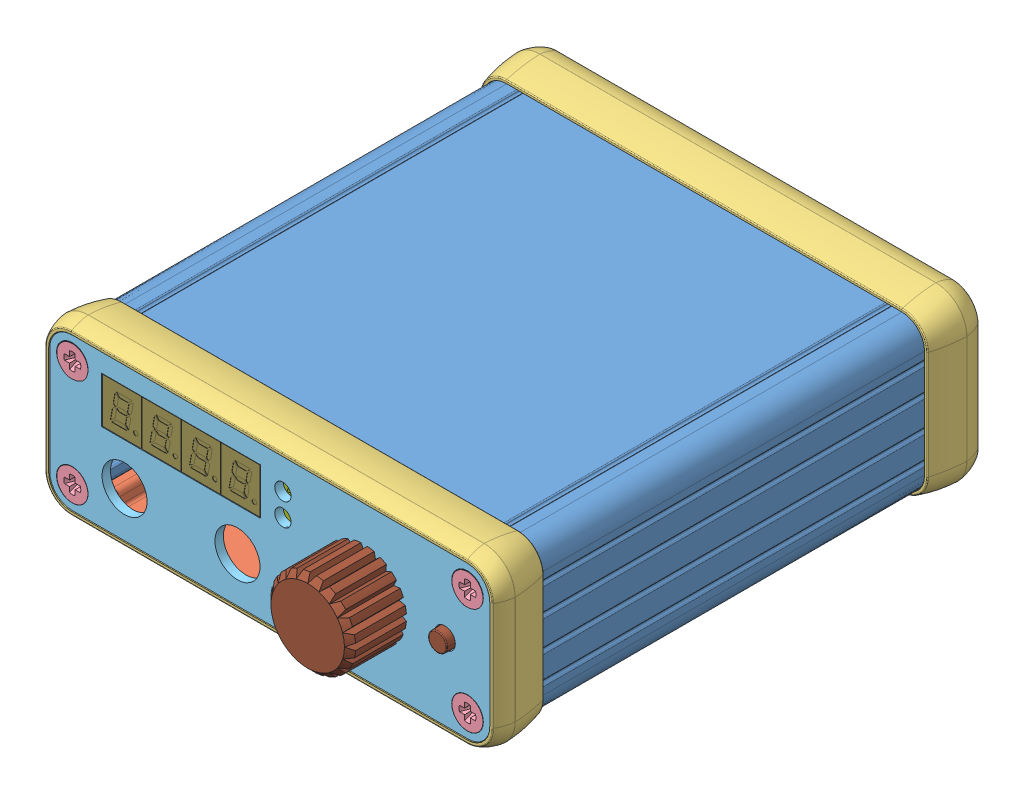
SolidWorks assembly Assembly_microbench_psu, configuration Standard. Lengths in mm. (continued)
Components (placement in the parent): (continued)
- main-board.step-1: main-board.step [Standard] at (-93.8915 -23.4474 -41.4) x (0 0 1) z (0 1 0) size (82.8 75 12.43) (continued)
  - C208.step-1: C208.step [Standard] at origin size (0.65 1.15 0.65) (continued)
    - 7876639952.step-1: 7876639952.step [Standard] at (30 50.9 0) x (0 1 0) z (0 0 1) size (1.15 0.65 0.65) (continued)
      - Terminal-3.step-1: Terminal-3.step [Standard] at (-0.575 -0.325 0) size (1.15 0.65 0.65)
        - Open CASCADE STEP translator 6.8 5.1.1-4.step-1: Open CASCADE STEP translator 6.8 5.1.1-4.step [Standard] at origin size (0.15 0.65 0.65)
        - Open CASCADE STEP translator 6.8 5.1.2-5.step-1: Open CASCADE STEP translator 6.8 5.1.2-5.step [Standard] at origin size (0.15 0.65 0.65)
      - Mid_Body-2.step-1: Mid_Body-2.step [Standard] at (-0.575 -0.325 0) size (0.85 0.65 0.65)
        - Open CASCADE STEP translator 6.8 5.2.1-6.step-1: Open CASCADE STEP translator 6.8 5.2.1-6.step [Standard] at origin size (0.85 0.65 0.65)
  - C207.step-1: C207.step [Standard] at origin size (0.65 1.15 0.65)
    - 7876647632.step-1: 7876647632.step [Standard] at (33.5 63.5 0) x (0 -1 0) z (0 0 1) size (1.15 0.65 0.65)
      - Terminal-6.step-1: Terminal-6.step [Standard] at (-0.575 -0.325 0) size (1.15 0.65 0.65)
        - Open CASCADE STEP translator 6.8 5.1.1-9.step-1: Open CASCADE STEP translator 6.8 5.1.1-9.step [Standard] at origin size (0.15 0.65 0.65)
        - Open CASCADE STEP translator 6.8 5.1.2-10.step-1: Open CASCADE STEP translator 6.8 5.1.2-10.step [Standard] at origin size (0.15 0.65 0.65)
      - Mid_Body-3.step-1: Mid_Body-3.step [Standard] at (-0.575 -0.325 0) size (0.85 0.65 0.65)
        - Open CASCADE STEP translator 6.8 5.2.1-11.step-1: Open CASCADE STEP translator 6.8 5.2.1-11.step [Standard] at origin size (0.85 0.65 0.65)
  - C206.step-1: C206.step [Standard] at origin size (0.65 1.15 0.65)
    - 7876647632.step-1: 7876647632.step [Standard] at (32.4 63.5 0) x (0 -1 0) z (0 0 1) size (1.15 0.65 0.65)
      - Terminal-6.step-1: Terminal-6.step [Standard] at (-0.575 -0.325 0) size (1.15 0.65 0.65)
        - Open CASCADE STEP translator 6.8 5.1.1-9.step-1: Open CASCADE STEP translator 6.8 5.1.1-9.step [Standard] at origin size (0.15 0.65 0.65)
        - Open CASCADE STEP translator 6.8 5.1.2-10.step-1: Open CASCADE STEP translator 6.8 5.1.2-10.step [Standard] at origin size (0.15 0.65 0.65)
      - Mid_Body-3.step-1: Mid_Body-3.step [Standard] at (-0.575 -0.325 0) size (0.85 0.65 0.65)
        - Open CASCADE STEP translator 6.8 5.2.1-11.step-1: Open CASCADE STEP translator 6.8 5.2.1-11.step [Standard] at origin size (0.85 0.65 0.65)
  - C205.step-1: C205.step [Standard] at origin size (0.65 1.15 0.65)
    - 7876639952.step-1: 7876639952.step [Standard] at (25.4 63.5 0) x (0 1 0) z (0 0 1) size (1.15 0.65 0.65)
      - Terminal-3.step-1: Terminal-3.step [Standard] at (-0.575 -0.325 0) size (1.15 0.65 0.65)
        - Open CASCADE STEP translator 6.8 5.1.1-4.step-1: Open CASCADE STEP translator 6.8 5.1.1-4.step [Standard] at origin size (0.15 0.65 0.65)
        - Open CASCADE STEP translator 6.8 5.1.2-5.step-1: Open CASCADE STEP translator 6.8 5.1.2-5.step [Standard] at origin size (0.15 0.65 0.65)
      - Mid_Body-2.step-1: Mid_Body-2.step [Standard] at (-0.575 -0.325 0) size (0.85 0.65 0.65)
        - Open CASCADE STEP translator 6.8 5.2.1-6.step-1: Open CASCADE STEP translator 6.8 5.2.1-6.step [Standard] at origin size (0.85 0.65 0.65)
  - C204.step-1: C204.step [Standard] at origin size (0.65 1.15 0.65)
    - 7876639952.step-1: 7876639952.step [Standard] at (30 62.5 0) x (0 1 0) z (0 0 1) size (1.15 0.65 0.65)
      - Terminal-3.step-1: Terminal-3.step [Standard] at (-0.575 -0.325 0) size (1.15 0.65 0.65)
        - Open CASCADE STEP translator 6.8 5.1.1-4.step-1: Open CASCADE STEP translator 6.8 5.1.1-4.step [Standard] at origin size (0.15 0.65 0.65)
        - Open CASCADE STEP translator 6.8 5.1.2-5.step-1: Open CASCADE STEP translator 6.8 5.1.2-5.step [Standard] at origin size (0.15 0.65 0.65)
      - Mid_Body-2.step-1: Mid_Body-2.step [Standard] at (-0.575 -0.325 0) size (0.85 0.65 0.65)
        - Open CASCADE STEP translator 6.8 5.2.1-6.step-1: Open CASCADE STEP translator 6.8 5.2.1-6.step [Standard] at origin size (0.85 0.65 0.65)
  - C203.step-1: C203.step [Standard] at origin size (0.65 1.15 0.65)
    - 7876647632.step-1: 7876647632.step [Standard] at (44.446 63.533 0) x (0 -1 0) z (0 0 1) size (1.15 0.65 0.65)
      - Terminal-6.step-1: Terminal-6.step [Standard] at (-0.575 -0.325 0) size (1.15 0.65 0.65)
        - Open CASCADE STEP translator 6.8 5.1.1-9.step-1: Open CASCADE STEP translator 6.8 5.1.1-9.step [Standard] at origin size (0.15 0.65 0.65)
        - Open CASCADE STEP translator 6.8 5.1.2-10.step-1: Open CASCADE STEP translator 6.8 5.1.2-10.step [Standard] at origin size (0.15 0.65 0.65)
      - Mid_Body-3.step-1: Mid_Body-3.step [Standard] at (-0.575 -0.325 0) size (0.85 0.65 0.65)
        - Open CASCADE STEP translator 6.8 5.2.1-11.step-1: Open CASCADE STEP translator 6.8 5.2.1-11.step [Standard] at origin size (0.85 0.65 0.65)
  - C202.step-1: C202.step [Standard] at origin size (0.65 1.15 0.65)
    - 7876647632.step-1: 7876647632.step [Standard] at (45.446 63.533 0) x (0 -1 0) z (0 0 1) size (1.15 0.65 0.65)
      - Terminal-6.step-1: Terminal-6.step [Standard] at (-0.575 -0.325 0) size (1.15 0.65 0.65)
        - Open CASCADE STEP translator 6.8 5.1.1-9.step-1: Open CASCADE STEP translator 6.8 5.1.1-9.step [Standard] at origin size (0.15 0.65 0.65)
        - Open CASCADE STEP translator 6.8 5.1.2-10.step-1: Open CASCADE STEP translator 6.8 5.1.2-10.step [Standard] at origin size (0.15 0.65 0.65)
      - Mid_Body-3.step-1: Mid_Body-3.step [Standard] at (-0.575 -0.325 0) size (0.85 0.65 0.65)
        - Open CASCADE STEP translator 6.8 5.2.1-11.step-1: Open CASCADE STEP translator 6.8 5.2.1-11.step [Standard] at origin size (0.85 0.65 0.65)
  - C201.step-1: C201.step [Standard] at origin size (0.65 1.15 0.65)
    - 7876639952.step-1: 7876639952.step [Standard] at (37.446 63.533 0) x (0 1 0) z (0 0 1) size (1.15 0.65 0.65)
      - Terminal-3.step-1: Terminal-3.step [Standard] at (-0.575 -0.325 0) size (1.15 0.65 0.65)
        - Open CASCADE STEP translator 6.8 5.1.1-4.step-1: Open CASCADE STEP translator 6.8 5.1.1-4.step [Standard] at origin size (0.15 0.65 0.65)
        - Open CASCADE STEP translator 6.8 5.1.2-5.step-1: Open CASCADE STEP translator 6.8 5.1.2-5.step [Standard] at origin size (0.15 0.65 0.65)
      - Mid_Body-2.step-1: Mid_Body-2.step [Standard] at (-0.575 -0.325 0) size (0.85 0.65 0.65)
        - Open CASCADE STEP translator 6.8 5.2.1-6.step-1: Open CASCADE STEP translator 6.8 5.2.1-6.step [Standard] at origin size (0.85 0.65 0.65)
  - C200.step-1: C200.step [Standard] at origin size (0.65 1.15 0.65)
    - 7876639952.step-1: 7876639952.step [Standard] at (42.046 62.533 0) x (0 1 0) z (0 0 1) size (1.15 0.65 0.65)
      - Terminal-3.step-1: Terminal-3.step [Standard] at (-0.575 -0.325 0) size (1.15 0.65 0.65)
        - Open CASCADE STEP translator 6.8 5.1.1-4.step-1: Open CASCADE STEP translator 6.8 5.1.1-4.step [Standard] at origin size (0.15 0.65 0.65)
        - Open CASCADE STEP translator 6.8 5.1.2-5.step-1: Open CASCADE STEP translator 6.8 5.1.2-5.step [Standard] at origin size (0.15 0.65 0.65)
      - Mid_Body-2.step-1: Mid_Body-2.step [Standard] at (-0.575 -0.325 0) size (0.85 0.65 0.65)
        - Open CASCADE STEP translator 6.8 5.2.1-6.step-1: Open CASCADE STEP translator 6.8 5.2.1-6.step [Standard] at origin size (0.85 0.65 0.65)
  - TR302.step-1: TR302.step [Standard] at origin size (3.05 2.64 1.12)
    - 7556043920.step-1: 7556043920.step [Standard] at (40.3 28.9 0) x (0 -1 0) z (0 0 1) size (2.64 3.04 1.12)
      - Body-4.step-1: Body-4.step [Standard] at (-0.7 -1.52 0) size (1.41 3.04 1.11)
        - Open CASCADE STEP translator 7.5 1.1.1-41.step-1: Open CASCADE STEP translator 7.5 1.1.1-41.step [Standard] at origin size (1.41 3.04 1.11)
      - Leader-42.step-1: Leader-42.step [Standard] at (-0.7 -0.95 0) x (-1 0 0) z (0 0 1) size (0.62 0.5 0.61)
      - Leader-42.step-2: Leader-42.step [Standard] at (-0.7 0.95 0) x (-1 0 0) z (0 0 1) size (0.62 0.5 0.61)
      - Leader-42.step-3: Leader-42.step [Standard] at (0.7 0 0) size (0.62 0.5 0.61)
  - TR300.step-1: TR300.step [Standard] at origin size (2.59 2.91 1.19)
    - 7556058560.step-1: 7556058560.step [Standard] at (36.1 21.2 0) size (2.59 2.91 1.19)
      - Body-6.step-1: Body-6.step [Standard] at (-0.8 -1.45 0) size (1.6 2.91 1.13)
        - Open CASCADE STEP translator 7.5 7.1.1-47.step-1: Open CASCADE STEP translator 7.5 7.1.1-47.step [Standard] at origin size (1.6 2.91 1.13)
      - Leader-48.step-1: Leader-48.step [Standard] at (-0.8 -0.95 0) x (-1 0 0) z (0 0 1) size (0.6 0.46 0.68)
      - Leader-48.step-2: Leader-48.step [Standard] at (-0.8 0 0) x (-1 0 0) z (0 0 1) size (0.6 0.46 0.68)
      - Leader-48.step-3: Leader-48.step [Standard] at (-0.8 0.95 0) x (-1 0 0) z (0 0 1) size (0.6 0.46 0.68)
      - Leader-48.step-4: Leader-48.step [Standard] at (0.8 -0.95 0) size (0.6 0.46 0.68)
      - Leader-48.step-5: Leader-48.step [Standard] at (0.8 0 0) size (0.6 0.46 0.68)
      - Leader-48.step-6: Leader-48.step [Standard] at (0.8 0.95 0) size (0.6 0.46 0.68)
  - TR301.step-1: TR301.step [Standard] at origin size (2.59 2.91 1.19)
    - 7556058560.step-1: 7556058560.step [Standard] at (41.6 21.2 0) size (2.59 2.91 1.19)
      - Body-6.step-1: Body-6.step [Standard] at (-0.8 -1.45 0) size (1.6 2.91 1.13)
        - Open CASCADE STEP translator 7.5 7.1.1-47.step-1: Open CASCADE STEP translator 7.5 7.1.1-47.step [Standard] at origin size (1.6 2.91 1.13)
      - Leader-48.step-1: Leader-48.step [Standard] at (-0.8 -0.95 0) x (-1 0 0) z (0 0 1) size (0.6 0.46 0.68)
      - Leader-48.step-2: Leader-48.step [Standard] at (-0.8 0 0) x (-1 0 0) z (0 0 1) size (0.6 0.46 0.68)
      - Leader-48.step-3: Leader-48.step [Standard] at (-0.8 0.95 0) x (-1 0 0) z (0 0 1) size (0.6 0.46 0.68)
      - Leader-48.step-4: Leader-48.step [Standard] at (0.8 -0.95 0) size (0.6 0.46 0.68)
      - Leader-48.step-5: Leader-48.step [Standard] at (0.8 0 0) size (0.6 0.46 0.68)
      - Leader-48.step-6: Leader-48.step [Standard] at (0.8 0.95 0) size (0.6 0.46 0.68)
  - R319.step-1: R319.step [Standard] at origin size (0.55 1.1 0.4)
    - 7876642432.step-1: 7876642432.step [Standard] at (51.7 41.9 0) x (0 1 0) z (0 0 1) size (1.1 0.55 0.4)
      - Terminal-12.step-1: Terminal-12.step [Standard] at (-0.55 -0.275 0) size (0.15 0.55 0.4)
        - Open CASCADE STEP translator 6.8 6.2.1-24.step-1: Open CASCADE STEP translator 6.8 6.2.1-24.step [Standard] at origin size (0.15 0.55 0.4)
      - Terminal-12.step-2: Terminal-12.step [Standard] at (0.55 0.275 0) x (-1 0 0) z (0 0 1) size (0.15 0.55 0.4)
        - Open CASCADE STEP translator 6.8 6.2.1-24.step-1: Open CASCADE STEP translator 6.8 6.2.1-24.step [Standard] at origin size (0.15 0.55 0.4)
      - Mid_Body-25.step-1: Mid_Body-25.step [Standard] at (-0.55 -0.275 0) size (1.02 0.55 0.32)
      - Mark-26.step-1: Mark-26.step [Standard] at (-0.4 -0.275 0.36) size (0.8 0.55 0.04)
  - R318.step-1: R318.step [Standard] at origin size (0.55 1.1 0.4)
    - 7876642992.step-1: 7876642992.step [Standard] at (51.7 40 0) x (0 -1 0) z (0 0 1) size (1.1 0.55 0.4)
      - Terminal-11.step-1: Terminal-11.step [Standard] at (-0.55 -0.275 0) size (0.15 0.55 0.4)
        - Open CASCADE STEP translator 6.8 6.2.1-21.step-1: Open CASCADE STEP translator 6.8 6.2.1-21.step [Standard] at origin size (0.15 0.55 0.4)
      - Terminal-11.step-2: Terminal-11.step [Standard] at (0.55 0.275 0) x (-1 0 0) z (0 0 1) size (0.15 0.55 0.4)
        - Open CASCADE STEP translator 6.8 6.2.1-21.step-1: Open CASCADE STEP translator 6.8 6.2.1-21.step [Standard] at origin size (0.15 0.55 0.4)
      - Mid_Body-22.step-1: Mid_Body-22.step [Standard] at (-0.55 -0.275 0) size (1.02 0.55 0.32)
      - Mark-23.step-1: Mark-23.step [Standard] at (-0.4 -0.275 0.36) size (0.8 0.55 0.04)
  - R317.step-1: R317.step [Standard] at origin size (0.55 1.1 0.4)
    - 7876642992.step-1: 7876642992.step [Standard] at (46 41.9 0) x (0 -1 0) z (0 0 1) size (1.1 0.55 0.4)
      - Terminal-11.step-1: Terminal-11.step [Standard] at (-0.55 -0.275 0) size (0.15 0.55 0.4)
        - Open CASCADE STEP translator 6.8 6.2.1-21.step-1: Open CASCADE STEP translator 6.8 6.2.1-21.step [Standard] at origin size (0.15 0.55 0.4)
      - Terminal-11.step-2: Terminal-11.step [Standard] at (0.55 0.275 0) x (-1 0 0) z (0 0 1) size (0.15 0.55 0.4)
        - Open CASCADE STEP translator 6.8 6.2.1-21.step-1: Open CASCADE STEP translator 6.8 6.2.1-21.step [Standard] at origin size (0.15 0.55 0.4)
      - Mid_Body-22.step-1: Mid_Body-22.step [Standard] at (-0.55 -0.275 0) size (1.02 0.55 0.32)
      - Mark-23.step-1: Mark-23.step [Standard] at (-0.4 -0.275 0.36) size (0.8 0.55 0.04)
  - R316.step-1: R316.step [Standard] at origin size (0.55 1.1 0.4)
    - 7876642992.step-1: 7876642992.step [Standard] at (46 40 0) x (0 -1 0) z (0 0 1) size (1.1 0.55 0.4)
      - Terminal-11.step-1: Terminal-11.step [Standard] at (-0.55 -0.275 0) size (0.15 0.55 0.4)
        - Open CASCADE STEP translator 6.8 6.2.1-21.step-1: Open CASCADE STEP translator 6.8 6.2.1-21.step [Standard] at origin size (0.15 0.55 0.4)
      - Terminal-11.step-2: Terminal-11.step [Standard] at (0.55 0.275 0) x (-1 0 0) z (0 0 1) size (0.15 0.55 0.4)
        - Open CASCADE STEP translator 6.8 6.2.1-21.step-1: Open CASCADE STEP translator 6.8 6.2.1-21.step [Standard] at origin size (0.15 0.55 0.4)
      - Mid_Body-22.step-1: Mid_Body-22.step [Standard] at (-0.55 -0.275 0) size (1.02 0.55 0.32)
      - Mark-23.step-1: Mark-23.step [Standard] at (-0.4 -0.275 0.36) size (0.8 0.55 0.04)
  - R315.step-1: R315.step [Standard] at origin size (0.55 1.1 0.4)
    - 7876642992.step-1: 7876642992.step [Standard] at (44.9 40 0) x (0 -1 0) z (0 0 1) size (1.1 0.55 0.4)
      - Terminal-11.step-1: Terminal-11.step [Standard] at (-0.55 -0.275 0) size (0.15 0.55 0.4)
        - Open CASCADE STEP translator 6.8 6.2.1-21.step-1: Open CASCADE STEP translator 6.8 6.2.1-21.step [Standard] at origin size (0.15 0.55 0.4)
      - Terminal-11.step-2: Terminal-11.step [Standard] at (0.55 0.275 0) x (-1 0 0) z (0 0 1) size (0.15 0.55 0.4)
        - Open CASCADE STEP translator 6.8 6.2.1-21.step-1: Open CASCADE STEP translator 6.8 6.2.1-21.step [Standard] at origin size (0.15 0.55 0.4)
      - Mid_Body-22.step-1: Mid_Body-22.step [Standard] at (-0.55 -0.275 0) size (1.02 0.55 0.32)
      - Mark-23.step-1: Mark-23.step [Standard] at (-0.4 -0.275 0.36) size (0.8 0.55 0.04)
  - R313.step-1: R313.step [Standard] at origin size (1.1 0.55 0.4)
    - 7876648592.step-1: 7876648592.step [Standard] at (26.9 9.1 0) x (-1 0 0) z (0 0 1) size (1.1 0.55 0.4)
      - Terminal.step-1: Terminal.step [Standard] at (-0.55 -0.275 0) size (0.15 0.55 0.4)
        - Open CASCADE STEP translator 6.8 6.2.1.step-1: Open CASCADE STEP translator 6.8 6.2.1.step [Standard] at origin size (0.15 0.55 0.4)
      - Terminal.step-2: Terminal.step [Standard] at (0.55 0.275 0) x (-1 0 0) z (0 0 1) size (0.15 0.55 0.4)
        - Open CASCADE STEP translator 6.8 6.2.1.step-1: Open CASCADE STEP translator 6.8 6.2.1.step [Standard] at origin size (0.15 0.55 0.4)
      - Mid_Body.step-1: Mid_Body.step [Standard] at (-0.55 -0.275 0) size (1.02 0.55 0.32)
      - Mark.step-1: Mark.step [Standard] at (-0.4 -0.275 0.36) size (0.8 0.55 0.04)
  - R312.step-1: R312.step [Standard] at origin size (1.1 0.55 0.4)
    - 7876648592.step-1: 7876648592.step [Standard] at (47.6 28.1 0) x (-1 0 0) z (0 0 1) size (1.1 0.55 0.4)
      - Terminal.step-1: Terminal.step [Standard] at (-0.55 -0.275 0) size (0.15 0.55 0.4)
        - Open CASCADE STEP translator 6.8 6.2.1.step-1: Open CASCADE STEP translator 6.8 6.2.1.step [Standard] at origin size (0.15 0.55 0.4)
      - Terminal.step-2: Terminal.step [Standard] at (0.55 0.275 0) x (-1 0 0) z (0 0 1) size (0.15 0.55 0.4)
        - Open CASCADE STEP translator 6.8 6.2.1.step-1: Open CASCADE STEP translator 6.8 6.2.1.step [Standard] at origin size (0.15 0.55 0.4)
      - Mid_Body.step-1: Mid_Body.step [Standard] at (-0.55 -0.275 0) size (1.02 0.55 0.32)
      - Mark.step-1: Mark.step [Standard] at (-0.4 -0.275 0.36) size (0.8 0.55 0.04)
  - R311.step-1: R311.step [Standard] at origin size (0.55 1.1 0.4)
    - 7876642432.step-1: 7876642432.step [Standard] at (47 25.5 0) x (0 1 0) z (0 0 1) size (1.1 0.55 0.4)
      - Terminal-12.step-1: Terminal-12.step [Standard] at (-0.55 -0.275 0) size (0.15 0.55 0.4)
        - Open CASCADE STEP translator 6.8 6.2.1-24.step-1: Open CASCADE STEP translator 6.8 6.2.1-24.step [Standard] at origin size (0.15 0.55 0.4)
      - Terminal-12.step-2: Terminal-12.step [Standard] at (0.55 0.275 0) x (-1 0 0) z (0 0 1) size (0.15 0.55 0.4)
        - Open CASCADE STEP translator 6.8 6.2.1-24.step-1: Open CASCADE STEP translator 6.8 6.2.1-24.step [Standard] at origin size (0.15 0.55 0.4)
      - Mid_Body-25.step-1: Mid_Body-25.step [Standard] at (-0.55 -0.275 0) size (1.02 0.55 0.32)
      - Mark-26.step-1: Mark-26.step [Standard] at (-0.4 -0.275 0.36) size (0.8 0.55 0.04)
  - R310.step-1: R310.step [Standard] at origin size (3.3 2.7 0.7)
    - 7556049520.step-1: 7556049520.step [Standard] at (49.5 9.5 0) x (1 0 0) z (0 0 1) size (3.3 2.7 0.7)
      - Terminal-17.step-1: Terminal-17.step [Standard] at (-1.65 -1.35 0) size (0.2 2.7 0.7)
        - Open CASCADE STEP translator 7.5 1.2.1-49.step-1: Open CASCADE STEP translator 7.5 1.2.1-49.step [Standard] at origin size (0.2 2.7 0.7)
      - Terminal-17.step-2: Terminal-17.step [Standard] at (1.65 1.35 0) x (-1 0 0) z (0 0 1) size (0.2 2.7 0.7)
        - Open CASCADE STEP translator 7.5 1.2.1-49.step-1: Open CASCADE STEP translator 7.5 1.2.1-49.step [Standard] at origin size (0.2 2.7 0.7)
      - Mid Body-50.step-1: Mid Body-50.step [Standard] at (-1.65 -1.35 0) size (3.16 2.7 0.56)
      - Mark-51.step-1: Mark-51.step [Standard] at (-1.45 -1.35 0.63) size (2.9 2.7 0.07)
  - R309.step-1: R309.step [Standard] at origin size (1.1 0.55 0.4)
    - 7556048720.step-1: 7556048720.step [Standard] at (47.6 29.2 0) x (1 0 0) z (0 0 1) size (1.1 0.55 0.4)
      - Terminal-10.step-1: Terminal-10.step [Standard] at (-0.55 -0.275 0) size (0.15 0.55 0.4)
        - Open CASCADE STEP translator 6.8 6.2.1-18.step-1: Open CASCADE STEP translator 6.8 6.2.1-18.step [Standard] at origin size (0.15 0.55 0.4)
      - Terminal-10.step-2: Terminal-10.step [Standard] at (0.55 0.275 0) x (-1 0 0) z (0 0 1) size (0.15 0.55 0.4)
        - Open CASCADE STEP translator 6.8 6.2.1-18.step-1: Open CASCADE STEP translator 6.8 6.2.1-18.step [Standard] at origin size (0.15 0.55 0.4)
      - Mid_Body-19.step-1: Mid_Body-19.step [Standard] at (-0.55 -0.275 0) size (1.02 0.55 0.32)
      - Mark-20.step-1: Mark-20.step [Standard] at (-0.4 -0.275 0.36) size (0.8 0.55 0.04)
  - R308.step-1: R308.step [Standard] at origin size (0.55 1.1 0.4)
    - 7876642992.step-1: 7876642992.step [Standard] at (44.9 29.8 0) x (0 -1 0) z (0 0 1) size (1.1 0.55 0.4)
      - Terminal-11.step-1: Terminal-11.step [Standard] at (-0.55 -0.275 0) size (0.15 0.55 0.4)
        - Open CASCADE STEP translator 6.8 6.2.1-21.step-1: Open CASCADE STEP translator 6.8 6.2.1-21.step [Standard] at origin size (0.15 0.55 0.4)
      - Terminal-11.step-2: Terminal-11.step [Standard] at (0.55 0.275 0) x (-1 0 0) z (0 0 1) size (0.15 0.55 0.4)
        - Open CASCADE STEP translator 6.8 6.2.1-21.step-1: Open CASCADE STEP translator 6.8 6.2.1-21.step [Standard] at origin size (0.15 0.55 0.4)
      - Mid_Body-22.step-1: Mid_Body-22.step [Standard] at (-0.55 -0.275 0) size (1.02 0.55 0.32)
      - Mark-23.step-1: Mark-23.step [Standard] at (-0.4 -0.275 0.36) size (0.8 0.55 0.04)
  - R306.step-1: R306.step [Standard] at origin size (1.1 0.55 0.4)
    - 7876648592.step-1: 7876648592.step [Standard] at (31.9 9.1 0) x (-1 0 0) z (0 0 1) size (1.1 0.55 0.4)
      - Terminal.step-1: Terminal.step [Standard] at (-0.55 -0.275 0) size (0.15 0.55 0.4)
        - Open CASCADE STEP translator 6.8 6.2.1.step-1: Open CASCADE STEP translator 6.8 6.2.1.step [Standard] at origin size (0.15 0.55 0.4)
      - Terminal.step-2: Terminal.step [Standard] at (0.55 0.275 0) x (-1 0 0) z (0 0 1) size (0.15 0.55 0.4)
        - Open CASCADE STEP translator 6.8 6.2.1.step-1: Open CASCADE STEP translator 6.8 6.2.1.step [Standard] at origin size (0.15 0.55 0.4)
      - Mid_Body.step-1: Mid_Body.step [Standard] at (-0.55 -0.275 0) size (1.02 0.55 0.32)
      - Mark.step-1: Mark.step [Standard] at (-0.4 -0.275 0.36) size (0.8 0.55 0.04)
  - R305.step-1: R305.step [Standard] at origin size (0.55 1.1 0.4)
    - 7876642992.step-1: 7876642992.step [Standard] at (39.4 32.1 0) x (0 -1 0) z (0 0 1) size (1.1 0.55 0.4)
      - Terminal-11.step-1: Terminal-11.step [Standard] at (-0.55 -0.275 0) size (0.15 0.55 0.4)
        - Open CASCADE STEP translator 6.8 6.2.1-21.step-1: Open CASCADE STEP translator 6.8 6.2.1-21.step [Standard] at origin size (0.15 0.55 0.4)
      - Terminal-11.step-2: Terminal-11.step [Standard] at (0.55 0.275 0) x (-1 0 0) z (0 0 1) size (0.15 0.55 0.4)
        - Open CASCADE STEP translator 6.8 6.2.1-21.step-1: Open CASCADE STEP translator 6.8 6.2.1-21.step [Standard] at origin size (0.15 0.55 0.4)
      - Mid_Body-22.step-1: Mid_Body-22.step [Standard] at (-0.55 -0.275 0) size (1.02 0.55 0.32)
      - Mark-23.step-1: Mark-23.step [Standard] at (-0.4 -0.275 0.36) size (0.8 0.55 0.04)
  - R304.step-1: R304.step [Standard] at origin size (0.55 1.1 0.4)
    - 7876642432.step-1: 7876642432.step [Standard] at (42.6 27.9 0) x (0 1 0) z (0 0 1) size (1.1 0.55 0.4)
      - Terminal-12.step-1: Terminal-12.step [Standard] at (-0.55 -0.275 0) size (0.15 0.55 0.4)
        - Open CASCADE STEP translator 6.8 6.2.1-24.step-1: Open CASCADE STEP translator 6.8 6.2.1-24.step [Standard] at origin size (0.15 0.55 0.4)
      - Terminal-12.step-2: Terminal-12.step [Standard] at (0.55 0.275 0) x (-1 0 0) z (0 0 1) size (0.15 0.55 0.4)
        - Open CASCADE STEP translator 6.8 6.2.1-24.step-1: Open CASCADE STEP translator 6.8 6.2.1-24.step [Standard] at origin size (0.15 0.55 0.4)
      - Mid_Body-25.step-1: Mid_Body-25.step [Standard] at (-0.55 -0.275 0) size (1.02 0.55 0.32)
      - Mark-26.step-1: Mark-26.step [Standard] at (-0.4 -0.275 0.36) size (0.8 0.55 0.04)
  - R303.step-1: R303.step [Standard] at origin size (0.55 1.1 0.4)
    - 7876642992.step-1: 7876642992.step [Standard] at (43.9 29.8 0) x (0 -1 0) z (0 0 1) size (1.1 0.55 0.4)
      - Terminal-11.step-1: Terminal-11.step [Standard] at (-0.55 -0.275 0) size (0.15 0.55 0.4)
        - Open CASCADE STEP translator 6.8 6.2.1-21.step-1: Open CASCADE STEP translator 6.8 6.2.1-21.step [Standard] at origin size (0.15 0.55 0.4)
      - Terminal-11.step-2: Terminal-11.step [Standard] at (0.55 0.275 0) x (-1 0 0) z (0 0 1) size (0.15 0.55 0.4)
        - Open CASCADE STEP translator 6.8 6.2.1-21.step-1: Open CASCADE STEP translator 6.8 6.2.1-21.step [Standard] at origin size (0.15 0.55 0.4)
      - Mid_Body-22.step-1: Mid_Body-22.step [Standard] at (-0.55 -0.275 0) size (1.02 0.55 0.32)
      - Mark-23.step-1: Mark-23.step [Standard] at (-0.4 -0.275 0.36) size (0.8 0.55 0.04)
  - R302.step-1: R302.step [Standard] at origin size (3.3 2.7 0.7)
    - 7556049520.step-1: 7556049520.step [Standard] at (49.5 13.5 0) x (1 0 0) z (0 0 1) size (3.3 2.7 0.7)
      - Terminal-17.step-1: Terminal-17.step [Standard] at (-1.65 -1.35 0) size (0.2 2.7 0.7)
        - Open CASCADE STEP translator 7.5 1.2.1-49.step-1: Open CASCADE STEP translator 7.5 1.2.1-49.step [Standard] at origin size (0.2 2.7 0.7)
      - Terminal-17.step-2: Terminal-17.step [Standard] at (1.65 1.35 0) x (-1 0 0) z (0 0 1) size (0.2 2.7 0.7)
        - Open CASCADE STEP translator 7.5 1.2.1-49.step-1: Open CASCADE STEP translator 7.5 1.2.1-49.step [Standard] at origin size (0.2 2.7 0.7)
      - Mid Body-50.step-1: Mid Body-50.step [Standard] at (-1.65 -1.35 0) size (3.16 2.7 0.56)
      - Mark-51.step-1: Mark-51.step [Standard] at (-1.45 -1.35 0.63) size (2.9 2.7 0.07)
  - R301.step-1: R301.step [Standard] at origin size (0.55 1.1 0.4)
    - 7876642432.step-1: 7876642432.step [Standard] at (44.1 24 0) x (0 1 0) z (0 0 1) size (1.1 0.55 0.4)
      - Terminal-12.step-1: Terminal-12.step [Standard] at (-0.55 -0.275 0) size (0.15 0.55 0.4)
        - Open CASCADE STEP translator 6.8 6.2.1-24.step-1: Open CASCADE STEP translator 6.8 6.2.1-24.step [Standard] at origin size (0.15 0.55 0.4)
      - Terminal-12.step-2: Terminal-12.step [Standard] at (0.55 0.275 0) x (-1 0 0) z (0 0 1) size (0.15 0.55 0.4)
        - Open CASCADE STEP translator 6.8 6.2.1-24.step-1: Open CASCADE STEP translator 6.8 6.2.1-24.step [Standard] at origin size (0.15 0.55 0.4)
      - Mid_Body-25.step-1: Mid_Body-25.step [Standard] at (-0.55 -0.275 0) size (1.02 0.55 0.32)
      - Mark-26.step-1: Mark-26.step [Standard] at (-0.4 -0.275 0.36) size (0.8 0.55 0.04)
  - R300.step-1: R300.step [Standard] at origin size (0.55 1.1 0.4)
    - 7876642432.step-1: 7876642432.step [Standard] at (42.9 24 0) x (0 1 0) z (0 0 1) size (1.1 0.55 0.4)
      - Terminal-12.step-1: Terminal-12.step [Standard] at (-0.55 -0.275 0) size (0.15 0.55 0.4)
        - Open CASCADE STEP translator 6.8 6.2.1-24.step-1: Open CASCADE STEP translator 6.8 6.2.1-24.step [Standard] at origin size (0.15 0.55 0.4)
      - Terminal-12.step-2: Terminal-12.step [Standard] at (0.55 0.275 0) x (-1 0 0) z (0 0 1) size (0.15 0.55 0.4)
        - Open CASCADE STEP translator 6.8 6.2.1-24.step-1: Open CASCADE STEP translator 6.8 6.2.1-24.step [Standard] at origin size (0.15 0.55 0.4)
      - Mid_Body-25.step-1: Mid_Body-25.step [Standard] at (-0.55 -0.275 0) size (1.02 0.55 0.32)
      - Mark-26.step-1: Mark-26.step [Standard] at (-0.4 -0.275 0.36) size (0.8 0.55 0.04)
  - IC309.step-1: IC309.step [Standard] at origin size (2.8 2.9 1.45)
    - 7556044960.step-1: 7556044960.step [Standard] at (54.4 44.6 0) size (2.8 2.91 1.45)
      - Body-7.step-1: Body-7.step [Standard] at (-0.8 -1.45 0) size (1.6 2.91 1.45)
        - Open CASCADE STEP translator 7.5 1.1.1-52.step-1: Open CASCADE STEP translator 7.5 1.1.1-52.step [Standard] at origin size (1.6 2.91 1.45)
      - Leader-53.step-1: Leader-53.step [Standard] at (-0.8 -0.95 0) x (-1 0 0) z (0 0 1) size (0.6 0.51 0.78)
      - Leader-53.step-2: Leader-53.step [Standard] at (-0.8 0 0) x (-1 0 0) z (0 0 1) size (0.6 0.51 0.78)
      - Leader-53.step-3: Leader-53.step [Standard] at (-0.8 0.95 0) x (-1 0 0) z (0 0 1) size (0.6 0.51 0.78)
      - Leader-53.step-4: Leader-53.step [Standard] at (0.8 -0.95 0) size (0.6 0.51 0.78)
      - Leader-53.step-5: Leader-53.step [Standard] at (0.8 0.95 0) size (0.6 0.51 0.78)
  - IC308.step-1: IC308.step [Standard] at origin size (2.3 2.01 1.1)
    - 7556047200.step-1: 7556047200.step [Standard] at (54.1 41.6 0) x (1 0 0) z (0 0 1) size (2.3 2 1.1)
      - Body-8.step-1: Body-8.step [Standard] at (-0.625 -1 0) size (1.25 2 1.1)
        - Open CASCADE STEP translator 7.5 4.1.1.step-1: Open CASCADE STEP translator 7.5 4.1.1.step [Standard] at origin size (1.25 2 1.1)
      - Leader-54.step-1: Leader-54.step [Standard] at (-0.625 -0.65 0) x (-1 0 0) z (0 0 1) size (0.53 0.4 0.6)
      - Leader-54.step-2: Leader-54.step [Standard] at (-0.625 0 0) x (-1 0 0) z (0 0 1) size (0.53 0.4 0.6)
      - Leader-54.step-3: Leader-54.step [Standard] at (-0.625 0.65 0) x (-1 0 0) z (0 0 1) size (0.53 0.4 0.6)
      - Leader-54.step-4: Leader-54.step [Standard] at (0.625 -0.65 0) size (0.53 0.4 0.6)
      - Leader-54.step-5: Leader-54.step [Standard] at (0.625 0.65 0) size (0.53 0.4 0.6)
  - IC301.step-1: IC301.step [Standard] at origin size (2.1 2.1 0.8)
    - 7556047680.step-1: 7556047680.step [Standard] at (44.8 26.4 0) x (1 0 0) z (0 0 1) size (2.1 2.1 0.8)
      - Body-9.step-1: Body-9.step [Standard] at (-1.05 -1.05 0) size (2.1 2.1 0.8)
        - Open CASCADE STEP translator 7.5 1.2.1-55.step-1: Open CASCADE STEP translator 7.5 1.2.1-55.step [Standard] at origin size (2.1 2.1 0.8)
      - Pin Shape-2.step-1: Pin Shape-2.step [Standard] at (-1.05 -0.91 0) size (0.4 0.32 0.2)
        - Open CASCADE STEP translator 7.5 1.4.1-56.step-1: Open CASCADE STEP translator 7.5 1.4.1-56.step [Standard] at origin size (0.4 0.32 0.2)
      - Pin Shape-2.step-2: Pin Shape-2.step [Standard] at (-1.05 -0.41 0) size (0.4 0.32 0.2)
        - Open CASCADE STEP translator 7.5 1.4.1-56.step-1: Open CASCADE STEP translator 7.5 1.4.1-56.step [Standard] at origin size (0.4 0.32 0.2)
      - Pin Shape-2.step-3: Pin Shape-2.step [Standard] at (-1.05 0.09 0) size (0.4 0.32 0.2)
        - Open CASCADE STEP translator 7.5 1.4.1-56.step-1: Open CASCADE STEP translator 7.5 1.4.1-56.step [Standard] at origin size (0.4 0.32 0.2)
      - Pin Shape-2.step-4: Pin Shape-2.step [Standard] at (-1.05 0.59 0) size (0.4 0.32 0.2)
        - Open CASCADE STEP translator 7.5 1.4.1-56.step-1: Open CASCADE STEP translator 7.5 1.4.1-56.step [Standard] at origin size (0.4 0.32 0.2)
      - Pin Shape-2.step-5: Pin Shape-2.step [Standard] at (1.05 -0.59 0) x (-1 0 0) z (0 0 1) size (0.4 0.32 0.2)
        - Open CASCADE STEP translator 7.5 1.4.1-56.step-1: Open CASCADE STEP translator 7.5 1.4.1-56.step [Standard] at origin size (0.4 0.32 0.2)
      - Pin Shape-2.step-6: Pin Shape-2.step [Standard] at (1.05 -0.09 0) x (-1 0 0) z (0 0 1) size (0.4 0.32 0.2)
        - Open CASCADE STEP translator 7.5 1.4.1-56.step-1: Open CASCADE STEP translator 7.5 1.4.1-56.step [Standard] at origin size (0.4 0.32 0.2)
      - Pin Shape-2.step-7: Pin Shape-2.step [Standard] at (1.05 0.41 0) x (-1 0 0) z (0 0 1) size (0.4 0.32 0.2)
        - Open CASCADE STEP translator 7.5 1.4.1-56.step-1: Open CASCADE STEP translator 7.5 1.4.1-56.step [Standard] at origin size (0.4 0.32 0.2)
      - Pin Shape-2.step-8: Pin Shape-2.step [Standard] at (1.05 0.91 0) x (-1 0 0) z (0 0 1) size (0.4 0.32 0.2)
        - Open CASCADE STEP translator 7.5 1.4.1-56.step-1: Open CASCADE STEP translator 7.5 1.4.1-56.step [Standard] at origin size (0.4 0.32 0.2)
      - Open CASCADE STEP translator 7.5 1.1-57.step-1: Open CASCADE STEP translator 7.5 1.1-57.step [Standard] at (-1.05 -1.05 0) size (0.27 0.27 0.01)
      - Thermal Shape-58.step-1: Thermal Shape-58.step [Standard] at (-0.45 -0.8 -0.001) size (0.9 1.6 0)
  - D300.step-1: D300.step [Standard] at origin size (2.81 5.1 1.1)
    - SODFL510X110-2N.step-1: SODFL510X110-2N.step [Standard] at (46.8 18.5 0) x (0 1 0) z (0 0 1) size (5.1 2.81 1.1)
      - Body-10.step-1: Body-10.step [Standard] at (-2.3 -1.4 0) size (4.6 2.8 1.1)
        - Open CASCADE STEP translator 6.8 15.1.1.step-1: Open CASCADE STEP translator 6.8 15.1.1.step [Standard] at origin size (4.6 2.8 1.1)
      - lead.step-1: lead.step [Standard] at (-2.55 -0.725 0) size (0.9 1.45 0.2)
      - lead.step-2: lead.step [Standard] at (2.55 0.725 0) x (-1 0 0) z (0 0 1) size (0.9 1.45 0.2)
  - C319.step-1: C319.step [Standard] at origin size (1.15 0.65 0.65)
    - 7556052240.step-1: 7556052240.step [Standard] at (53.2 39.7 0) x (-1 0 0) z (0 0 1) size (1.15 0.65 0.65)
      - Terminal-1.step-1: Terminal-1.step [Standard] at (-0.575 -0.325 0) size (1.15 0.65 0.65)
        - Open CASCADE STEP translator 6.8 5.1.1.step-1: Open CASCADE STEP translator 6.8 5.1.1.step [Standard] at origin size (0.15 0.65 0.65)
        - Open CASCADE STEP translator 6.8 5.1.2.step-1: Open CASCADE STEP translator 6.8 5.1.2.step [Standard] at origin size (0.15 0.65 0.65)
      - Mid_Body-0.step-1: Mid_Body-0.step [Standard] at (-0.575 -0.325 0) size (0.85 0.65 0.65)
        - Open CASCADE STEP translator 6.8 5.2.1.step-1: Open CASCADE STEP translator 6.8 5.2.1.step [Standard] at origin size (0.85 0.65 0.65)
  - C318.step-1: C318.step [Standard] at origin size (0.65 1.15 0.65)
    - 7876647632.step-1: 7876647632.step [Standard] at (51.7 43.8 0) x (0 -1 0) z (0 0 1) size (1.15 0.65 0.65)
      - Terminal-6.step-1: Terminal-6.step [Standard] at (-0.575 -0.325 0) size (1.15 0.65 0.65)
        - Open CASCADE STEP translator 6.8 5.1.1-9.step-1: Open CASCADE STEP translator 6.8 5.1.1-9.step [Standard] at origin size (0.15 0.65 0.65)
        - Open CASCADE STEP translator 6.8 5.1.2-10.step-1: Open CASCADE STEP translator 6.8 5.1.2-10.step [Standard] at origin size (0.15 0.65 0.65)
      - Mid_Body-3.step-1: Mid_Body-3.step [Standard] at (-0.575 -0.325 0) size (0.85 0.65 0.65)
        - Open CASCADE STEP translator 6.8 5.2.1-11.step-1: Open CASCADE STEP translator 6.8 5.2.1-11.step [Standard] at origin size (0.85 0.65 0.65)
  - C317.step-1: C317.step [Standard] at origin size (0.65 1.15 0.65)
    - 7876639952.step-1: 7876639952.step [Standard] at (51.7 45.7 0) x (0 1 0) z (0 0 1) size (1.15 0.65 0.65)
      - Terminal-3.step-1: Terminal-3.step [Standard] at (-0.575 -0.325 0) size (1.15 0.65 0.65)
        - Open CASCADE STEP translator 6.8 5.1.1-4.step-1: Open CASCADE STEP translator 6.8 5.1.1-4.step [Standard] at origin size (0.15 0.65 0.65)
        - Open CASCADE STEP translator 6.8 5.1.2-5.step-1: Open CASCADE STEP translator 6.8 5.1.2-5.step [Standard] at origin size (0.15 0.65 0.65)
      - Mid_Body-2.step-1: Mid_Body-2.step [Standard] at (-0.575 -0.325 0) size (0.85 0.65 0.65)
        - Open CASCADE STEP translator 6.8 5.2.1-6.step-1: Open CASCADE STEP translator 6.8 5.2.1-6.step [Standard] at origin size (0.85 0.65 0.65)
  - C316.step-1: C316.step [Standard] at origin size (0.65 1.15 0.65)
    - 7876639952.step-1: 7876639952.step [Standard] at (56.4 41.9 0) x (0 1 0) z (0 0 1) size (1.15 0.65 0.65)
      - Terminal-3.step-1: Terminal-3.step [Standard] at (-0.575 -0.325 0) size (1.15 0.65 0.65)
        - Open CASCADE STEP translator 6.8 5.1.1-4.step-1: Open CASCADE STEP translator 6.8 5.1.1-4.step [Standard] at origin size (0.15 0.65 0.65)
        - Open CASCADE STEP translator 6.8 5.1.2-5.step-1: Open CASCADE STEP translator 6.8 5.1.2-5.step [Standard] at origin size (0.15 0.65 0.65)
      - Mid_Body-2.step-1: Mid_Body-2.step [Standard] at (-0.575 -0.325 0) size (0.85 0.65 0.65)
        - Open CASCADE STEP translator 6.8 5.2.1-6.step-1: Open CASCADE STEP translator 6.8 5.2.1-6.step [Standard] at origin size (0.85 0.65 0.65)
  - C307.step-1: C307.step [Standard] at origin size (1.15 0.65 0.65)
    - 7556050560.step-1: 7556050560.step [Standard] at (47.6 27 0) x (1 0 0) z (0 0 1) size (1.15 0.65 0.65)
      - Terminal-2.step-1: Terminal-2.step [Standard] at (-0.575 -0.325 0) size (1.15 0.65 0.65)
        - Open CASCADE STEP translator 6.8 5.1.1-1.step-1: Open CASCADE STEP translator 6.8 5.1.1-1.step [Standard] at origin size (0.15 0.65 0.65)
        - Open CASCADE STEP translator 6.8 5.1.2-2.step-1: Open CASCADE STEP translator 6.8 5.1.2-2.step [Standard] at origin size (0.15 0.65 0.65)
      - Mid_Body-1.step-1: Mid_Body-1.step [Standard] at (-0.575 -0.325 0) size (0.85 0.65 0.65)
        - Open CASCADE STEP translator 6.8 5.2.1-3.step-1: Open CASCADE STEP translator 6.8 5.2.1-3.step [Standard] at origin size (0.85 0.65 0.65)
  - C305.step-1: C305.step [Standard] at origin size (0.65 1.15 0.65)
    - 7876639952.step-1: 7876639952.step [Standard] at (46 30.4 0) x (0 1 0) z (0 0 1) size (1.15 0.65 0.65)
      - Terminal-3.step-1: Terminal-3.step [Standard] at (-0.575 -0.325 0) size (1.15 0.65 0.65)
        - Open CASCADE STEP translator 6.8 5.1.1-4.step-1: Open CASCADE STEP translator 6.8 5.1.1-4.step [Standard] at origin size (0.15 0.65 0.65)
        - Open CASCADE STEP translator 6.8 5.1.2-5.step-1: Open CASCADE STEP translator 6.8 5.1.2-5.step [Standard] at origin size (0.15 0.65 0.65)
      - Mid_Body-2.step-1: Mid_Body-2.step [Standard] at (-0.575 -0.325 0) size (0.85 0.65 0.65)
        - Open CASCADE STEP translator 6.8 5.2.1-6.step-1: Open CASCADE STEP translator 6.8 5.2.1-6.step [Standard] at origin size (0.85 0.65 0.65)
  - C304.step-1: C304.step [Standard] at origin size (0.65 1.15 0.65)
    - 7876639952.step-1: 7876639952.step [Standard] at (42.9 29.8 0) x (0 1 0) z (0 0 1) size (1.15 0.65 0.65)
      - Terminal-3.step-1: Terminal-3.step [Standard] at (-0.575 -0.325 0) size (1.15 0.65 0.65)
        - Open CASCADE STEP translator 6.8 5.1.1-4.step-1: Open CASCADE STEP translator 6.8 5.1.1-4.step [Standard] at origin size (0.15 0.65 0.65)
        - Open CASCADE STEP translator 6.8 5.1.2-5.step-1: Open CASCADE STEP translator 6.8 5.1.2-5.step [Standard] at origin size (0.15 0.65 0.65)
      - Mid_Body-2.step-1: Mid_Body-2.step [Standard] at (-0.575 -0.325 0) size (0.85 0.65 0.65)
        - Open CASCADE STEP translator 6.8 5.2.1-6.step-1: Open CASCADE STEP translator 6.8 5.2.1-6.step [Standard] at origin size (0.85 0.65 0.65)
  - C300.step-1: C300.step [Standard] at origin size (1.15 0.65 0.65)
    - 7556050560.step-1: 7556050560.step [Standard] at (45 28.3 0) x (1 0 0) z (0 0 1) size (1.15 0.65 0.65)
      - Terminal-2.step-1: Terminal-2.step [Standard] at (-0.575 -0.325 0) size (1.15 0.65 0.65)
        - Open CASCADE STEP translator 6.8 5.1.1-1.step-1: Open CASCADE STEP translator 6.8 5.1.1-1.step [Standard] at origin size (0.15 0.65 0.65)
        - Open CASCADE STEP translator 6.8 5.1.2-2.step-1: Open CASCADE STEP translator 6.8 5.1.2-2.step [Standard] at origin size (0.15 0.65 0.65)
      - Mid_Body-1.step-1: Mid_Body-1.step [Standard] at (-0.575 -0.325 0) size (0.85 0.65 0.65)
        - Open CASCADE STEP translator 6.8 5.2.1-3.step-1: Open CASCADE STEP translator 6.8 5.2.1-3.step [Standard] at origin size (0.85 0.65 0.65)
  - R314.step-1: R314.step [Standard] at origin size (0.55 1.1 0.4)
    - 7876642992.step-1: 7876642992.step [Standard] at (39.2 41.3 0) x (0 -1 0) z (0 0 1) size (1.1 0.55 0.4)
      - Terminal-11.step-1: Terminal-11.step [Standard] at (-0.55 -0.275 0) size (0.15 0.55 0.4)
        - Open CASCADE STEP translator 6.8 6.2.1-21.step-1: Open CASCADE STEP translator 6.8 6.2.1-21.step [Standard] at origin size (0.15 0.55 0.4)
      - Terminal-11.step-2: Terminal-11.step [Standard] at (0.55 0.275 0) x (-1 0 0) z (0 0 1) size (0.15 0.55 0.4)
        - Open CASCADE STEP translator 6.8 6.2.1-21.step-1: Open CASCADE STEP translator 6.8 6.2.1-21.step [Standard] at origin size (0.15 0.55 0.4)
      - Mid_Body-22.step-1: Mid_Body-22.step [Standard] at (-0.55 -0.275 0) size (1.02 0.55 0.32)
      - Mark-23.step-1: Mark-23.step [Standard] at (-0.4 -0.275 0.36) size (0.8 0.55 0.04)
  - IC307.step-1: IC307.step [Standard] at origin size (2.8 2.9 1.45)
    - 7556044960.step-1: 7556044960.step [Standard] at (48.6 44.6 0) size (2.8 2.91 1.45)
      - Body-7.step-1: Body-7.step [Standard] at (-0.8 -1.45 0) size (1.6 2.91 1.45)
        - Open CASCADE STEP translator 7.5 1.1.1-52.step-1: Open CASCADE STEP translator 7.5 1.1.1-52.step [Standard] at origin size (1.6 2.91 1.45)
      - Leader-53.step-1: Leader-53.step [Standard] at (-0.8 -0.95 0) x (-1 0 0) z (0 0 1) size (0.6 0.51 0.78)
      - Leader-53.step-2: Leader-53.step [Standard] at (-0.8 0 0) x (-1 0 0) z (0 0 1) size (0.6 0.51 0.78)
      - Leader-53.step-3: Leader-53.step [Standard] at (-0.8 0.95 0) x (-1 0 0) z (0 0 1) size (0.6 0.51 0.78)
      - Leader-53.step-4: Leader-53.step [Standard] at (0.8 -0.95 0) size (0.6 0.51 0.78)
      - Leader-53.step-5: Leader-53.step [Standard] at (0.8 0.95 0) size (0.6 0.51 0.78)
  - IC306.step-1: IC306.step [Standard] at origin size (2.3 2 1.1)
    - 7556049760.step-1: 7556049760.step [Standard] at (48.3 41.6 0) size (2.3 2 1.1)
      - Body-11.step-1: Body-11.step [Standard] at (-0.625 -1 0) size (1.25 2 1.1)
        - Open CASCADE STEP translator 7.5 4.1.1-59.step-1: Open CASCADE STEP translator 7.5 4.1.1-59.step [Standard] at origin size (1.25 2 1.1)
      - Leader-60.step-1: Leader-60.step [Standard] at (-0.625 -0.65 0) x (-1 0 0) z (0 0 1) size (0.53 0.4 0.6)
      - Leader-60.step-2: Leader-60.step [Standard] at (-0.625 0 0) x (-1 0 0) z (0 0 1) size (0.53 0.4 0.6)
      - Leader-60.step-3: Leader-60.step [Standard] at (-0.625 0.65 0) x (-1 0 0) z (0 0 1) size (0.53 0.4 0.6)
      - Leader-60.step-4: Leader-60.step [Standard] at (0.625 -0.65 0) size (0.53 0.4 0.6)
      - Leader-60.step-5: Leader-60.step [Standard] at (0.625 0.65 0) size (0.53 0.4 0.6)
  - IC305.step-1: IC305.step [Standard] at origin size (2.8 2.9 1.45)
    - 7556044960.step-1: 7556044960.step [Standard] at (41.9 44.6 0) size (2.8 2.91 1.45)
      - Body-7.step-1: Body-7.step [Standard] at (-0.8 -1.45 0) size (1.6 2.91 1.45)
        - Open CASCADE STEP translator 7.5 1.1.1-52.step-1: Open CASCADE STEP translator 7.5 1.1.1-52.step [Standard] at origin size (1.6 2.91 1.45)
